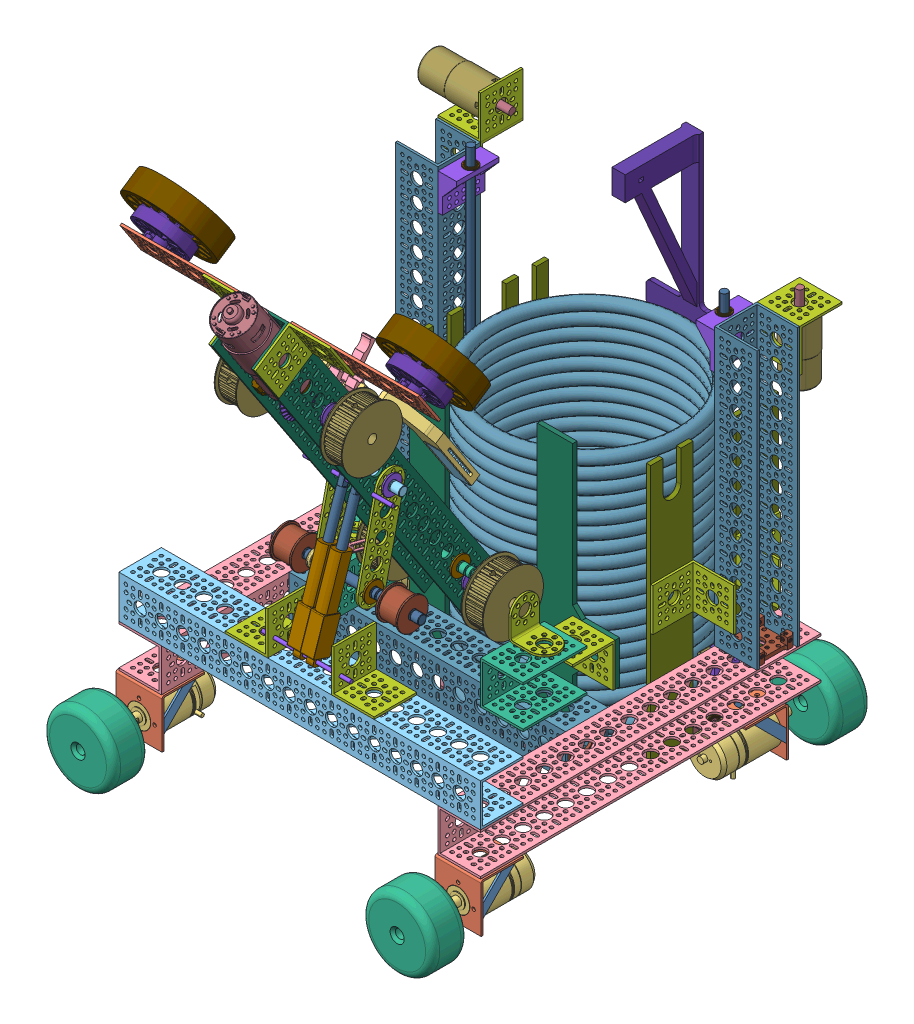
SolidWorks assembly 底座3.5, configuration 默认. Lengths in mm.
Overall size (466.71 646.3 560.79).
166 component instances, 54 part files, 189 mates.
Components (placement in the parent):
- 电机连接支架-5: 电机连接支架 [默认] at (-222.052 128.3372 691.3695) x (0 0 1) z (-1 0 0) size (48 54.5 52)
  - 小兔电机连接支架02-1: 小兔电机连接支架02 [默认] at (-18.8303 11.0829 24.6066) size (36.21 36.21 2)
  - 小兔电机连接支架02-2: 小兔电机连接支架02 [默认] at (-18.8303 11.0829 -25.3934) size (36.21 36.21 2)
  - 小兔电机连接支架-1: 小兔电机连接支架 [默认] at (17.3829 -18.9171 0.6066) size (48 54.5 52)
- 电机连接支架-6: 电机连接支架 [默认] at (137.948 128.3372 691.3695) x (0 0 1) z (-1 0 0) size (48 54.5 52)
  - 小兔电机连接支架02-1: 小兔电机连接支架02 [默认] at (-18.8303 11.0829 24.6066) size (36.21 36.21 2)
  - 小兔电机连接支架02-2: 小兔电机连接支架02 [默认] at (-18.8303 11.0829 -25.3934) size (36.21 36.21 2)
  - 小兔电机连接支架-1: 小兔电机连接支架 [默认] at (17.3829 -18.9171 0.6066) size (48 54.5 52)
- 3508无刷电机带减速箱（00）-5: 3508无刷电机带减速箱（00） [默认] at (137.3414 109.4201 681.1524) x (-1 0 0) z (0 -1 0) size (42 98.3 47)
- 3508无刷电机带减速箱（00）-7: 3508无刷电机带减速箱（00） [默认] at (-222.6586 109.4201 681.1524) x (0 -1 0) z (1 0 0) size (42 98.3 47)
- 384mm-U型梁-1: 384mm-U型梁 [默认] at (-201.1586 165.4201 709.5024) x (0 -1 0) z (1 0 0) size (48 384 48)
- 384mm-U型梁-2: 384mm-U型梁 [默认] at (115.8414 165.4201 709.5024) x (0 1 0) z (-1 0 0) size (48 384 48)
- 408mm-U型梁-10: 408mm-U型梁 [默认] at (161.3414 213.4201 707.0024) x (0 1 0) z (0 0 1) size (48 408 48)
- 电机连接支架-7: 电机连接支架 [默认] at (136.7348 128.3372 383.6353) x (0 0 -1) z (1 0 0) size (48 54.5 52)
  - 小兔电机连接支架02-1: 小兔电机连接支架02 [默认] at (-18.8303 11.0829 24.6066) size (36.21 36.21 2)
  - 小兔电机连接支架02-2: 小兔电机连接支架02 [默认] at (-18.8303 11.0829 -25.3934) size (36.21 36.21 2)
  - 小兔电机连接支架-1: 小兔电机连接支架 [默认] at (17.3829 -18.9171 0.6066) size (48 54.5 52)
- 3508无刷电机带减速箱（00）-8: 3508无刷电机带减速箱（00） [默认] at (137.3414 109.4201 393.8524) x (1 0 0) z (0 -1 0) size (42 98.3 47)
- 电机连接支架-8: 电机连接支架 [默认] at (-223.2652 128.3372 383.6353) x (0 0 -1) z (1 0 0) size (48 54.5 52)
  - 小兔电机连接支架02-1: 小兔电机连接支架02 [默认] at (-18.8303 11.0829 24.6066) size (36.21 36.21 2)
  - 小兔电机连接支架02-2: 小兔电机连接支架02 [默认] at (-18.8303 11.0829 -25.3934) size (36.21 36.21 2)
  - 小兔电机连接支架-1: 小兔电机连接支架 [默认] at (17.3829 -18.9171 0.6066) size (48 54.5 52)
- 3508无刷电机带减速箱（00）-9: 3508无刷电机带减速箱（00） [默认] at (-222.6586 109.4201 393.8524) x (1 0 0) z (0 -1 0) size (42 98.3 47)
- 麦轮（临时）-1: 麦轮（临时） [默认] at (-222.6586 109.4201 324.5024) x (0 0 -1) z (0.996866 -0.079106 0) size (40 80 80)
- 麦轮（临时）-2: 麦轮（临时） [默认] at (137.3414 109.4201 324.5024) x (0 0 -1) z (0.923265 -0.384164 0) size (40 80 80)
- 麦轮（临时）-3: 麦轮（临时） [默认] at (137.3414 109.4201 779.5024) x (0 0 -1) z (0.99707 -0.076496 0) size (40 80 80)
- 麦轮（临时）-4: 麦轮（临时） [默认] at (-222.6586 109.4201 779.5024) x (0 0 -1) z (0.996866 -0.079106 0) size (40 80 80)
- 48x48-L形支架-3: 48x48-L形支架 [默认] at (-81.1586 261.4201 709.5024) x (0 -1 0) z (1 0 0) size (48 48 48)
- 48x48-L形支架-4: 48x48-L形支架 [默认] at (-4.1586 261.4201 661.5024) x (0 -1 0) z (-1 0 0) size (48 48 48)
- 升降轴-1: 升降轴 [默认] at (-92.6586 252.9349 701.0171) x (1 0 0) z (0 0.719401 -0.694595) size (100 4 4)
- 电动推杆01-1: 电动推杆01 [默认] at (-54.1586 252.9349 701.0171) x (1 0 0) z (0 -0.94837 0.317167) size (15 20 103)
- 电动推杆01-2: 电动推杆01 [默认] at (-39.1586 252.9349 701.0171) x (1 0 0) z (0 -0.94837 0.317167) size (15 20 103)
- 电动推杆2-1: 电动推杆2 [默认] at (-35.1586 340.9577 671.5793) x (-1 0 0) z (0 -0.317167 -0.94837) size (9 66 9)
- 电动推杆2-2: 电动推杆2 [默认] at (-50.1586 340.9577 671.5793) x (-1 0 0) z (0 -0.317167 -0.94837) size (9 66 9)
- 升降轴-2: 升降轴 [默认] at (-94.6586 399.2825 652.0735) x (1 0 0) z (0 -0.677442 -0.735576) size (100 4 4)
- 电机转向座-9: 电机转向座 [默认] at (137.3414 189.4201 373.5024) x (0 0 -1) z (1 0 0) size (43.24 12.23 43.24)
- 电机转向座-12: 电机转向座 [默认] at (-222.6586 189.4201 373.5024) x (0 0 -1) z (1 0 0) size (43.24 12.23 43.24)
- 48x48-L形支架-17: 48x48-L形支架 [默认] at (161.3414 477.4201 347.0024) x (0 1 0) z (0 0 1) size (48 48 48)
- 48x48-L形支架-18: 48x48-L形支架 [默认] at (-198.6586 477.4201 347.0024) x (0 1 0) z (0 0 1) size (48 48 48)
- 一级摩擦轮电机01-2: 一级摩擦轮电机01 [默认] at (137.3414 425.6201 325.5024) x (0.035714 0 0.999362) z (-0.999362 0 0.035714) size (36 73.3 36)
- 一级摩擦轮电机02-2: 一级摩擦轮电机02 [默认] at (137.3414 495.9201 325.5024) x (-0.966562 0 0.256432) z (-0.256432 0 -0.966562) size (8 20 8)
- 312mm-U型梁-7: 312mm-U型梁 [默认] at (-198.6586 186.9201 541.5024) x (0 0 1) z (0 1 0) size (48 312 48)
- 电机转向座-13: 电机转向座 [默认] at (113.3414 165.4201 541.5024) x (0 0 -1) z (0 1 0) size (43.24 12.23 43.24)
- 总装-2: 总装 [默认] at (-93.0333 217.2746 993.3883) x (-0.999953 0.009266 0.002717) z (0 0.281421 -0.959585) size (409.26 486.07 201.86)
  - 432mm-U型梁-1: 432mm-U型梁 [默认] at (-52.5612 -100.8788 473.6792) x (0.999953 -0.009656 0) z (0.002854 0.295554 0.955322) size (48 432 48)
  - 发射法兰1-2: 发射法兰1 [默认] at (95.3037 298.6557 389.1988) x (0.597612 -0.766469 0.235342) z (0.801781 0.57024 -0.178814) size (30 11 30)
  - 发射无刷电机-2: 发射无刷电机 [默认] at (95.2101 288.9616 357.8642) x (-0.009225 -0.955277 0.295568) z (-0.999953 0.009656 0) size (58.5 35.4 58.5)
  - 摩擦轮-2: 摩擦轮 [默认] at (94.6021 282.6082 387.0905) x (-0.954993 -0.28256 0.09027) z (-0.002854 -0.295554 -0.955322) size (96 96 24)
    - 摩擦轮.STEP-1: 摩擦轮.STEP [默认] at origin size (96 96 24)
      - 3613-0014-0096 Rubber.STEP-1: 3613-0014-0096 Rubber.STEP [默认] at (-5.0141 13.8433 -6.759) size (96 96 24)
      - 3613-0014-0096 Core.STEP-1: 3613-0014-0096 Core.STEP [默认] at (-5.0141 13.8433 -6.759) x (1 0 0) z (0 -1 0) size (35.2 24 35.2)
  - 5孔平板-2: 5孔平板 [默认] at (119.072 274.5458 384.7583) x (0.002854 0.295554 0.955322) z (-0.009225 -0.955277 0.295568) size (2.5 144 43)
  - 48x48-L形支架-2: 48x48-L形支架 [默认] at (-22.5815 259.3374 339.6418) x (0.002854 0.295554 0.955322) z (-0.999953 0.009656 0) size (48 48 48)
  - 装配体3-2: 装配体3 [默认] at (-128.0634 200.7559 231.0431) x (0.002854 0.295554 0.955322) z (0.999953 -0.009656 0) size (95.3 120.73 180.37)
    - 发射法兰1-1: 发射法兰1 [默认] at (180.6617 -48.8364 -65.5887) x (0 1 0) z (0 0 1) size (30 11 30)
    - 发射无刷电机-1: 发射无刷电机 [默认] at (147.8617 -48.8364 -65.5887) x (0 -1 0) z (0 0 1) size (58.5 35.4 58.5)
    - 摩擦轮-1: 摩擦轮 [默认] at (173.9027 -63.5495 -65.0421) x (0 -0.305413 0.95222) z (-1 0 0) size (96 96 24)
      - 摩擦轮.STEP-1: 摩擦轮.STEP [默认] at origin size (96 96 24)
        - 3613-0014-0096 Rubber.STEP-1: 3613-0014-0096 Rubber.STEP [默认] at (-5.0141 13.8433 -6.759) size (96 96 24)
        - 3613-0014-0096 Core.STEP-1: 3613-0014-0096 Core.STEP [默认] at (-5.0141 13.8433 -6.759) x (1 0 0) z (0 -1 0) size (35.2 24 35.2)
    - 5孔平板-1: 5孔平板 [默认] at (169.3617 -70.3364 -89.5887) x (1 0 0) z (0 -1 0) size (2.5 144 43)
    - 48x48-L形支架-1: 48x48-L形支架 [默认] at (121.3617 -72.8364 51.9113) size (48 48 48)
  - 2306-4008-0014 assembly-1: 2306-4008-0014 assembly [默认] at (-186.8079 96.5973 629.512) x (0 0.597801 0.801645) z (-0.223733 -0.781323 0.582647)
  - 不锈钢花篮螺丝-02-1: 不锈钢花篮螺丝-02 [默认] at (-13.6983 -11.7016 355.7521) x (-0.999953 0.009656 0) z (0.008275 0.856874 0.51546) size (4.31 46.15 18.3)
  - 花篮螺丝-1: 花篮螺丝 [默认] at (-71.9313 -35.5534 412.0649) x (0.008275 0.856874 0.51546) z (0.999953 -0.009656 0) size (18.3 77.15 7)
    - 不锈钢花篮螺丝-01-1: 不锈钢花篮螺丝-01 [默认] at (-8.1072 20.254 58) size (9 58 7)
    - 不锈钢花篮螺丝-02-1: 不锈钢花篮螺丝-02 [默认] at (-8.1072 29.254 58) x (0 0 1) z (1 0 0) size (4.31 46.15 18.3)
  - 张紧固定轴2-1: 张紧固定轴2 [默认] at (-22.3528 75.9048 396.3908) x (-0.999953 0.009656 0) z (0.003811 0.394647 0.918825) size (81 10 10)
  - 张紧固定轴3-1: 张紧固定轴3 [默认] at (-78.1786 -61.1289 438.9525) x (0.999953 -0.009656 0) z (-0.003263 -0.337938 -0.941163) size (90 10 10)
  - 圆角孔板5孔(1)-1: 圆角孔板5孔(1) [默认] at (-25.1629 -7.9825 349.7537) x (0.00844 0.874027 0.485803) z (-0.004691 -0.485781 0.874068) size (128 2.5 32)
  - 铜套-1: 铜套 [默认] at (-22.3528 75.9048 396.3908) x (-0.999953 0.009656 0) z (0.009537 0.98756 -0.156954) size (10 22 22)
  - 铜套1-5: 铜套1 [默认] at (-78.1786 -61.1289 438.9525) x (0.999953 -0.009656 0) z (0 0 1) size (10 22 22)
  - 铜套1-6: 铜套1 [默认] at (-26.181 -61.631 438.9525) x (-0.999953 0.009656 0) z (0 0 1) size (10 22 22)
  - 张紧固定轴(中)-1: 张紧固定轴(中) [默认] at (-77.6605 -7.4756 349.7537) x (0.999953 -0.009656 0) z (0.007656 0.792843 0.609378) size (166 10 10)
  - 张紧轮1-3: 张紧轮1 [默认] at (-4.1639 -8.1853 349.7537) x (0.999953 -0.009656 0) z (-0.000665 -0.068842 0.997627) size (25 35 35)
  - 铜套1-8: 铜套1 [默认] at (-23.163 -8.0018 349.7537) x (-0.999953 0.009656 0) z (-0.007437 -0.770127 -0.637848) size (10 22 22)
  - 同步轮四十齿(1)-1: 同步轮四十齿(1) [默认] at (20.0954 -85.0067 446.0461) x (0.009586 0.99273 -0.119983) z (0.001159 0.119977 0.992776) size (68 25 68)
  - 同步轮四十齿(1)-2: 同步轮四十齿(1) [默认] at (22.7522 190.1132 360.9227) x (0.004551 0.471293 -0.881965) z (0.008516 0.881924 0.471315) size (68 25 68)
  - 同步轮四十齿(1)-3: 同步轮四十齿(1) [默认] at (-99.1635 -83.855 446.0461) x (0.009623 0.996484 -0.083229) z (0.000804 0.083225 0.99653) size (68 25 68)
  - 同步轮四十齿(1)-4: 同步轮四十齿(1) [默认] at (-96.5067 191.2649 360.9227) x (0.00965 0.999279 0.036717) z (-0.000355 -0.036715 0.999326) size (68 25 68)
  - 皮带电机装配体-3: 皮带电机装配体 [默认] at (17.3534 305.199 468.5412) x (0.009225 0.955277 -0.295568) z (0.002854 0.295554 0.955322) size (182.3 67.11 64.42)
    - 发射轮电机1-1: 发射轮电机1 [默认] at (-31.948 68.6302 -206.7966) size (148.5 67.11 64.42)
    - 3204-0002-0002 assembly-1: 3204-0002-0002 assembly [默认] at (-82.9257 129.4143 -179.1986) x (0 1 0) z (0 0 1) size (28.67 52.38 42.6)
      - 2306-4008-0014 assembly(2)-1: 2306-4008-0014 assembly(2) [默认] at (-86.5036 -22.1715 14.0673) x (0 1 0) z (-0.223733 0 0.97465) size (15.4 23.81 24.42)
        - 2306-4008-0014-1: 2306-4008-0014 [默认] at (-4.2928 -28.4802 22.5212) size (15.32 23.81 24.42)
        - 2306-4008-0014 clamp-1: 2306-4008-0014 clamp [默认] at (-4.2932 -28.4802 22.5212) size (9.55 8.86 18.72)
        - 2800-0004-0012_90128A207-1: 2800-0004-0012_90128A207 [默认] at (-8.9015 -37.2302 16.6212) x (0.549526 0 0.835476) z (0 -1 0) size (7 7 16.17)
        - 2800-0004-0012_90128A207-2: 2800-0004-0012_90128A207 [默认] at (-8.9015 -37.2302 28.4212) x (0.549526 0 -0.835476) z (0 -1 0) size (7 7 16.17)
      - 2307-0014-0028-1: 2307-0014-0028 [默认] at (-76.6728 -4.8452 42.3896) size (6.41 42.6 42.6)
    - 齿轮组法兰-1: 齿轮组法兰 [默认] at (-78.0805 56.1302 -136.809) x (0 1 0) z (0 0 1) size (12 30 30) (hidden)
    - 电机转向座1-1: 电机转向座1 [默认] at (-41.0801 65.9902 -136.809) x (0 0 -1) z (0 -1 0) size (43.24 12.23 43.24)
  - 张紧轮1-4: 张紧轮1 [默认] at (-124.1583 -7.0266 349.7537) x (0.999953 -0.009656 0) z (-0.001384 -0.14335 0.989671) size (25 35 35)
  - 滑轨9-1: 滑轨9 [默认] at (-54.9831 -92.7733 473.7957) x (0.999953 -0.009656 0) z (-0.009225 -0.955277 0.295568) size (5 3.7 400)
  - 钩子总装修改-1: 钩子总装修改 [默认] at (-51.1458 183.362 391.6503) x (0.999953 -0.009656 0) z (-0.009225 -0.955277 0.295568) size (146 51.58 153.26)
    - 滑块1-1: 滑块1 [默认] at (1.3294 2.8515 16) size (12 5 16)
    - 滑块座1-1: 滑块座1 [默认] at (-33.6706 2.8515 4) size (146 18 125)
    - 抓钩1-1: 抓钩1 [默认] at (6.3294 45.8627 -7.2454) x (0 -0.424487 0.905434) z (0 -0.905434 -0.424487) size (35.49 30 38.32)
    - 移动块-1: 移动块 [默认] at (62.3294 9.8515 101.6458) x (0 0 1) z (-1 0 0) size (60 11 18)
    - 移动块-2: 移动块 [默认] at (-59.6706 9.8515 101.6458) x (0 0 1) z (-1 0 0) size (60 11 18)
  - 铜套-2: 铜套 [默认] at (-75.7432 191.0643 360.9227) x (0.999953 -0.009656 0) z (0 0 1) size (10 22 22)
  - 铜套-3: 铜套 [默认] at (-23.7457 190.5622 360.9227) x (-0.999953 0.009656 0) z (-0.009078 -0.94012 -0.340724) size (10 22 22)
  - 铜套-4: 铜套 [默认] at (-78.4 -84.0555 446.0461) x (0.999953 -0.009656 0) z (0.000026 0.002689 0.999996) size (10 22 22)
  - 铜套-5: 铜套 [默认] at (-26.4024 -84.5576 446.0461) x (-0.999953 0.009656 0) z (-0.009078 -0.94012 -0.340724) size (10 22 22)
  - 铜套-6: 铜套 [默认] at (-79.3501 76.4552 396.3908) x (0.999953 -0.009656 0) z (0 0 1) size (10 22 22)
  - 圆角孔板5孔(1)-2: 圆角孔板5孔(1) [默认] at (-75.6606 -7.4949 349.7537) x (0.00844 0.874027 0.485803) z (-0.004691 -0.485781 0.874068) size (128 2.5 32)
  - 铜套1-9: 铜套1 [默认] at (-80.1604 -7.4514 349.7537) x (0.999953 -0.009656 0) z (0.003758 0.38916 -0.921163) size (10 22 22)
- 72mm-U型梁-5: 72mm-U型梁 [默认] at (43.8414 213.4201 517.5024) x (0 -1 0) z (-1 0 0) size (48 72 48)
- 72mm-U型梁-6: 72mm-U型梁 [默认] at (-129.1586 213.4201 517.5024) x (0 1 0) z (1 0 0) size (48 72 48)
- 圆角90°法兰-7: 圆角90°法兰 [默认] at (41.3414 237.4201 541.5024) x (1 0 0) z (0 -1 0) size (40 32 40)
- 圆角90°法兰-8: 圆角90°法兰 [默认] at (-126.6586 237.4201 541.5024) x (-1 0 0) z (0 -1 0) size (40 32 40)
- 轴承座-1: 轴承座 [Default] at (113.3414 492.4201 397.5024) x (-1 0 0) z (0 0 -1) size (21 41 48)
- 8-14轴承-7: 8-14轴承 [默认] at (100.3414 493.4201 373.5024) x (0.974446 0 0.224624) z (-0.224624 0 0.974446) size (15 5 15)
- 轴承座-2: 轴承座 [Default] at (113.3414 150.4201 349.5024) x (-1 0 0) z (0 0 1) size (21 41 48)
- 8-14轴承-8: 8-14轴承 [默认] at (100.3414 146.4201 373.5024) x (0.983901 0 0.178713) z (-0.178713 0 0.983901) size (15 5 15)
- 螺纹杆-3: 螺纹杆 [默认] at (100.3414 117.4201 373.5024) x (0.005803 0 0.999983) z (-0.999983 0 0.005803) size (8 400 8)
- 切边螺纹滑块-1: 切边螺纹滑块 [Default] at (100.3414 168.0411 373.5024) x (-1 0 0) z (0 0 1) size (10.2 15 22)
- 轴承座-3: 轴承座 [Default] at (-198.6586 492.4201 349.5024) size (21 41 48)
- 轴承座-4: 轴承座 [Default] at (-198.6586 150.4201 397.5024) x (1 0 0) z (0 0 -1) size (21 41 48)
- 8-14轴承-9: 8-14轴承 [默认] at (-185.6586 493.4201 373.5024) size (15 5 15)
- 8-14轴承-10: 8-14轴承 [默认] at (-185.6586 146.4201 373.5024) size (15 5 15)
- 螺纹杆-4: 螺纹杆 [默认] at (-185.6586 117.4201 373.5024) x (0.186577 0 0.98244) z (-0.98244 0 0.186577) size (8 400 8)
- 切边螺纹滑块-2: 切边螺纹滑块 [Default] at (-185.6586 168.0411 373.5024) x (-1 0 0) z (0 0 1) size (10.2 15 22)
- 转换块-1: 转换块 [Default] at (100.3414 158.0411 373.5024) x (0 0 1) z (-1 0 0) size (24 85 26)
- 转换块-2: 转换块 [Default] at (-185.6586 158.0411 373.5024) x (0 0 -1) z (1 0 0) size (24 85 26)
- 312mm-U型梁-8: 312mm-U型梁 [默认] at (115.8414 501.4201 373.5024) x (0 0 -1) z (-1 0 0) size (48 312 48)
- 312mm-U型梁-9: 312mm-U型梁 [默认] at (-201.1586 501.4201 373.5024) x (0 0 1) z (1 0 0) size (48 312 48)
- 8-14轴承-11: 8-14轴承 [默认] at (83.3414 90.0411 373.5024) x (0 0.99609 -0.088349) z (0 -0.088349 -0.99609) size (15 5 15)
- 8-14轴承-12: 8-14轴承 [默认] at (-168.6586 90.0411 373.5024) x (0 -0.55352 0.832836) z (0 -0.832836 -0.55352) size (15 5 15)
- 铲板-1: 铲板 [Default] at (-42.6586 74.7848 398.3468) x (-1 0 0) z (0 0.010285 -0.999947) size (262 29 178.51)
- 20个环-3: 20个环 [Default] at (-127.5441 -59.6219 226.4779) size (229.8 290.93 229.39)
  - 圆环-1: 圆环 [默认] at (-22.7884 145.7519 157.2951) size (228 14 228)
  - 圆环-2: 圆环 [默认] at (-23.1175 159.9955 157.1344) size (228 14 228)
  - 圆环-3: 圆环 [默认] at (-23.0314 188.5505 156.9811) size (228 14 228)
  - 圆环-4: 圆环 [默认] at (-22.9968 174.3685 156.6405) size (228 14 228)
  - 圆环-5: 圆环 [默认] at (-23.8175 218.055 156.8293) size (228 14 228)
  - 圆环-6: 圆环 [默认] at (-23.491 232.7117 157.4697) size (228 14 228)
  - 圆环-7: 圆环 [默认] at (-24.5846 203.4176 157.6394) size (228 14 228)
  - 圆环-8: 圆环 [默认] at (-22.9081 247.4608 157.3208) size (228 14 228)
  - 圆环-9: 圆环 [默认] at (-23.5661 364.5462 157.293) size (228 14 228)
  - 圆环-10: 圆环 [默认] at (-23.6099 320.9711 157.4866) size (228 14 228)
  - 圆环-11: 圆环 [默认] at (-23.6825 350.1705 157.5218) size (228 14 228)
  - 圆环-12: 圆环 [默认] at (-24.0088 276.7124 157.1259) size (228 14 228)
  - 圆环-13: 圆环 [默认] at (-23.8881 291.321 157.9228) size (228 14 228)
  - 圆环-14: 圆环 [默认] at (-23.6797 261.8797 158.031) size (228 14 228)
  - 圆环-15: 圆环 [默认] at (-24.0091 335.4434 157.9465) size (228 14 228)
  - 圆环-16: 圆环 [默认] at (-23.4562 306.0805 156.7976) size (228 14 228)
  - 圆环-17: 圆环 [默认] at (-24.0369 393.8042 157.2623) size (228 14 228)
  - 圆环-18: 圆环 [默认] at (-23.9162 408.195 157.1866) size (228 14 228)
  - 圆环-19: 圆环 [默认] at (-23.9606 379.2206 157.4915) size (228 14 228)
  - 圆环-20: 圆环 [默认] at (-23.698 422.6814 157.0029) size (228 14 228)
- 48x48-L形支架-20: 48x48-L形支架 [默认] at (-134.6586 232.4201 517.5024) x (0 0 -1) z (0 1 0) size (48 48 48)
- 前挡板-1: 前挡板 [Default] at (-94.6586 402.9201 493.5024) x (-1 0 0) z (0 0 -1) size (88 278 5)
- 48x48-L形支架-22: 48x48-L形支架 [默认] at (-198.6586 261.4201 400.0024) x (1 0 0) z (0 0 -1) size (48 48 48)
- 48x48-L形支架-23: 48x48-L形支架 [默认] at (-198.6586 213.4201 347.0024) size (48 48 48)
- 侧挡板-1: 侧挡板 [Default] at (-174.6586 77.4201 301.5024) x (0 0 1) z (1 0 0) size (48 300 5)
- 侧挡板-2: 侧挡板 [Default] at (-174.6586 77.4201 397.5024) x (0 0 1) z (1 0 0) size (48 300 5)
- 侧挡板-3: 侧挡板 [Default] at (84.3414 77.4201 301.5024) x (0 0 1) z (1 0 0) size (48 300 5)
- 侧挡板-4: 侧挡板 [Default] at (84.3414 77.4201 397.5024) x (0 0 1) z (1 0 0) size (48 300 5)
- 48x48-L形支架-24: 48x48-L形支架 [默认] at (91.8414 213.4201 325.5024) x (0 0 1) z (-1 0 0) size (48 48 48)
- 48x48-L形支架-25: 48x48-L形支架 [默认] at (113.3414 213.4201 400.0024) x (-1 0 0) z (0 0 -1) size (48 48 48)
- 48x48-L形支架-26: 48x48-L形支架 [默认] at (97.3414 232.4201 517.5024) x (0 0 -1) z (0 1 0) size (48 48 48)
- 前挡板-2: 前挡板 [Default] at (9.3414 402.9201 488.5024) size (88 278 5)
- 推板-1: 推板 [默认] at (-41.8089 369.725 264.6148) size (100 195 86)
- 一级摩擦轮电机02-3: 一级摩擦轮电机02 [默认] at (-206.7756 525.4201 325.5024) x (0 -0.907269 -0.420551) z (0 -0.420551 0.907269) size (8 20 8)
- 一级摩擦轮电机01-4: 一级摩擦轮电机01 [默认] at (-277.0756 525.4201 325.5024) x (0 -0.562838 0.826567) z (0 0.826567 0.562838) size (36 73.3 36)
- 48x48-L形支架-27: 48x48-L形支架 [默认] at (-201.1586 525.4201 349.5024) x (0 -1 0) z (1 0 0) size (48 48 48)
Mates (geometry in assembly coordinates):
- Coincident37: coincident anti-aligned: plane of 电机连接支架-5/小兔电机连接支架-1 through (-222.6586 109.4201 708.7524) normal (0 0 -1); plane of 3508无刷电机带减速箱（00）-7 through (-222.6586 96.4201 708.7524) normal (0 0 1)
- Concentric38: concentric aligned: cylinder of 电机连接支架-5/小兔电机连接支架-1 through (-222.6586 109.4201 710.7524) axis (0 0 -1) radius 13.25; cylinder of 3508无刷电机带减速箱（00）-7 through (-222.6586 109.4201 672.4524) axis (0 0 -1) radius 13
- Concentric39: concentric anti-aligned: cylinder of 电机连接支架-5/小兔电机连接支架-1 through (-222.6586 126.9201 710.7524) axis (0 0 -1) radius 2; cylinder of 3508无刷电机带减速箱（00）-7 through (-222.6586 126.9201 708.7524) axis (0 0 1) radius 1.65
- Coincident38: coincident anti-aligned: plane of 电机连接支架-6/小兔电机连接支架-1 through (137.3414 109.4201 708.7524) normal (0 0 -1); plane of 3508无刷电机带减速箱（00）-5 through (124.3414 109.4201 708.7524) normal (0 0 1)
- Concentric40: concentric aligned: cylinder of 电机连接支架-6/小兔电机连接支架-1 through (137.3414 109.4201 710.7524) axis (0 0 -1) radius 13.25; cylinder of 3508无刷电机带减速箱（00）-5 through (137.3414 109.4201 672.4524) axis (0 0 -1) radius 13
- Concentric41: concentric anti-aligned: cylinder of 电机连接支架-6/小兔电机连接支架-1 through (137.3414 126.9201 710.7524) axis (0 0 -1) radius 2; cylinder of 3508无刷电机带减速箱（00）-5 through (137.3414 126.9201 708.7524) axis (0 0 1) radius 1.65
- Concentric261: concentric anti-aligned: cylinder of 384mm-U型梁-2 through (137.3414 179.4201 685.5024) axis (0 1 0) radius 7; cylinder of 408mm-U型梁-10 through (137.3414 199.4201 685.5024) axis (0 -1 0) radius 7
- Concentric262: concentric anti-aligned: cylinder of 384mm-U型梁-1 through (-222.6586 179.4201 685.5024) axis (0 1 0) radius 7; cylinder of 408mm-U型梁-10 through (-222.6586 199.4201 685.5024) axis (0 -1 0) radius 7
- Coincident94: coincident aligned: plane of 384mm-U型梁-2 through (161.3414 186.9201 325.5024) normal (1 0 0); plane of 408mm-U型梁-10 through (161.3414 213.4201 707.0024) normal (1 0 0)
- Coincident95: coincident aligned: plane of 384mm-U型梁-1 through (-246.6586 186.9201 325.5024) normal (-1 0 0); plane of 408mm-U型梁-10 through (-246.6586 213.4201 707.0024) normal (-1 0 0)
- Coincident96: coincident anti-aligned: plane of 384mm-U型梁-1 through (-246.6586 189.4201 325.5024) normal (0 1 0); plane of 408mm-U型梁-10 through (-246.6586 189.4201 661.5024) normal (0 -1 0)
- Coincident97: coincident anti-aligned: plane of 384mm-U型梁-2 through (161.3414 189.4201 325.5024) normal (0 1 0); plane of 408mm-U型梁-10 through (-246.6586 189.4201 661.5024) normal (0 -1 0)
- Concentric267: concentric aligned: cylinder of 电机连接支架-7/小兔电机连接支架-1 through (137.3414 109.4201 364.2524) axis (0 0 1) radius 13.25; cylinder of 3508无刷电机带减速箱（00）-8 through (137.3414 109.4201 402.5524) axis (0 0 1) radius 13
- Coincident104: coincident anti-aligned: plane of 电机连接支架-7/小兔电机连接支架-1 through (137.3414 109.4201 366.2524) normal (0 0 1); plane of 3508无刷电机带减速箱（00）-8 through (150.3414 109.4201 366.2524) normal (0 0 -1)
- Concentric268: concentric anti-aligned: cylinder of 电机连接支架-7/小兔电机连接支架-1 through (137.3414 126.9201 364.2524) axis (0 0 1) radius 2; cylinder of 3508无刷电机带减速箱（00）-8 through (137.3414 126.9201 366.2524) axis (0 0 -1) radius 1.65
- Concentric269: concentric aligned: cylinder of 电机连接支架-8/小兔电机连接支架-1 through (-222.6586 109.4201 364.2524) axis (0 0 1) radius 13.25; cylinder of 3508无刷电机带减速箱（00）-9 through (-222.6586 109.4201 402.5524) axis (0 0 1) radius 13
- Coincident105: coincident anti-aligned: plane of 电机连接支架-8/小兔电机连接支架-1 through (-222.6586 109.4201 366.2524) normal (0 0 1); plane of 3508无刷电机带减速箱（00）-9 through (-209.6586 109.4201 366.2524) normal (0 0 -1)
- Concentric270: concentric anti-aligned: cylinder of 电机连接支架-8/小兔电机连接支架-1 through (-222.6586 126.9201 364.2524) axis (0 0 1) radius 2; cylinder of 3508无刷电机带减速箱（00）-9 through (-222.6586 126.9201 366.2524) axis (0 0 -1) radius 1.65
- Concentric271: concentric anti-aligned: cylinder of 电机连接支架-6/小兔电机连接支架-1 through (137.3414 86.9201 685.5024) axis (0 1 0) radius 7; cylinder of 384mm-U型梁-2 through (137.3414 151.4201 685.5024) axis (0 -1 0) radius 7
- Coincident106: coincident anti-aligned: plane of 电机连接支架-6/小兔电机连接支架-1 through (163.3414 141.4201 662.7524) normal (0 1 0); plane of 384mm-U型梁-2 through (161.3414 141.4201 325.5024) normal (0 -1 0)
- Concentric272: concentric anti-aligned: cylinder of 电机连接支架-6/小兔电机连接支架-1 through (153.3414 86.9201 701.5024) axis (0 1 0) radius 2; cylinder of 384mm-U型梁-2 through (153.3414 151.4201 701.5024) axis (0 -1 0) radius 2
- Concentric273: concentric anti-aligned: cylinder of 电机连接支架-5/小兔电机连接支架-1 through (-222.6586 86.9201 685.5024) axis (0 1 0) radius 7; cylinder of 384mm-U型梁-1 through (-222.6586 151.4201 685.5024) axis (0 -1 0) radius 7
- Coincident107: coincident anti-aligned: plane of 电机连接支架-5/小兔电机连接支架-1 through (-196.6586 141.4201 662.7524) normal (0 1 0); plane of 384mm-U型梁-1 through (-246.6586 141.4201 325.5024) normal (0 -1 0)
- Concentric274: concentric anti-aligned: cylinder of 电机连接支架-5/小兔电机连接支架-1 through (-206.6586 86.9201 701.5024) axis (0 1 0) radius 2; cylinder of 384mm-U型梁-1 through (-206.6586 151.4201 701.5024) axis (0 -1 0) radius 2
- Coincident108: coincident anti-aligned: plane of 384mm-U型梁-2 through (161.3414 141.4201 325.5024) normal (0 -1 0); plane of 电机连接支架-7/小兔电机连接支架-1 through (111.3414 141.4201 412.2524) normal (0 1 0)
- Concentric276: concentric anti-aligned: cylinder of 384mm-U型梁-2 through (153.3414 151.4201 373.5024) axis (0 -1 0) radius 2; cylinder of 电机连接支架-7/小兔电机连接支架-1 through (153.3414 86.9201 373.5024) axis (0 1 0) radius 2
- Concentric277: concentric anti-aligned: cylinder of 384mm-U型梁-2 through (121.3414 151.4201 373.5024) axis (0 -1 0) radius 2; cylinder of 电机连接支架-7/小兔电机连接支架-1 through (121.3414 86.9201 373.5024) axis (0 1 0) radius 2
- Coincident109: coincident anti-aligned: plane of 384mm-U型梁-1 through (-246.6586 141.4201 325.5024) normal (0 -1 0); plane of 电机连接支架-8/小兔电机连接支架-1 through (-248.6586 141.4201 412.2524) normal (0 1 0)
- Concentric278: concentric anti-aligned: cylinder of 384mm-U型梁-1 through (-238.6586 151.4201 373.5024) axis (0 -1 0) radius 2; cylinder of 电机连接支架-8/小兔电机连接支架-1 through (-238.6586 86.9201 373.5024) axis (0 1 0) radius 2
- Concentric279: concentric anti-aligned: cylinder of 384mm-U型梁-1 through (-206.6586 151.4201 373.5024) axis (0 -1 0) radius 2; cylinder of 电机连接支架-8/小兔电机连接支架-1 through (-206.6586 86.9201 373.5024) axis (0 1 0) radius 2
- Concentric280: concentric anti-aligned: cylinder of 3508无刷电机带减速箱（00）-9 through (-222.6586 109.4201 402.5524) axis (0 0 1) radius 5; cylinder of 麦轮（临时）-1 through (-222.6586 109.4201 324.5024) axis (0 0 -1) radius 5
- Distance1: distance = 1 mm anti-aligned: plane of 麦轮（临时）-1 through (-222.6586 109.4201 324.5024) normal (0 0 1); plane of 384mm-U型梁-1 through (-201.1586 165.4201 325.5024) normal (0 0 -1)
- Concentric281: concentric anti-aligned: cylinder of 3508无刷电机带减速箱（00）-8 through (137.3414 109.4201 402.5524) axis (0 0 1) radius 5; cylinder of 麦轮（临时）-2 through (137.3414 109.4201 324.5024) axis (0 0 -1) radius 5
- Distance2: distance = 1 mm anti-aligned: plane of 384mm-U型梁-2 through (115.8414 165.4201 325.5024) normal (0 0 -1); plane of 麦轮（临时）-2 through (137.3414 109.4201 324.5024) normal (0 0 1)
- Concentric282: concentric aligned: cylinder of 3508无刷电机带减速箱（00）-5 through (137.3414 109.4201 672.4524) axis (0 0 -1) radius 5; cylinder of 麦轮（临时）-3 through (137.3414 109.4201 779.5024) axis (0 0 -1) radius 5
- Distance3: distance = 495 mm anti-aligned: plane of 麦轮（临时）-3 through (137.3414 109.4201 779.5024) normal (0 0 1); plane of 麦轮（临时）-2 through (137.3414 109.4201 284.5024) normal (0 0 -1)
- Concentric283: concentric aligned: cylinder of 3508无刷电机带减速箱（00）-7 through (-222.6586 109.4201 672.4524) axis (0 0 -1) radius 5; cylinder of 麦轮（临时）-4 through (-222.6586 109.4201 779.5024) axis (0 0 -1) radius 5
- Distance4: distance = 495 mm anti-aligned: plane of 麦轮（临时）-4 through (-222.6586 109.4201 779.5024) normal (0 0 1); plane of 麦轮（临时）-1 through (-222.6586 109.4201 284.5024) normal (0 0 -1)
- Coincident120: coincident anti-aligned: plane of 408mm-U型梁-10 through (-246.6586 237.4201 661.5024) normal (0 1 0); plane of 48x48-L形支架-3 through (-126.6586 237.4201 661.5024) normal (0 -1 0)
- Concentric309: concentric anti-aligned: cylinder of 408mm-U型梁-10 through (-102.6586 227.4201 685.5024) axis (0 1 0) radius 7; cylinder of 48x48-L形支架-3 through (-102.6586 247.4201 685.5024) axis (0 -1 0) radius 7
- Concentric310: concentric anti-aligned: cylinder of 408mm-U型梁-10 through (-118.6586 227.4201 669.5024) axis (0 1 0) radius 2; cylinder of 48x48-L形支架-3 through (-118.6586 247.4201 669.5024) axis (0 -1 0) radius 2
- Concentric311: concentric anti-aligned: cylinder of 408mm-U型梁-10 through (17.3414 227.4201 685.5024) axis (0 1 0) radius 7; cylinder of 48x48-L形支架-4 through (17.3414 247.4201 685.5024) axis (0 -1 0) radius 7
- Coincident121: coincident anti-aligned: plane of 408mm-U型梁-10 through (-246.6586 237.4201 661.5024) normal (0 1 0); plane of 48x48-L形支架-4 through (41.3414 237.4201 709.5024) normal (0 -1 0)
- Concentric312: concentric anti-aligned: cylinder of 408mm-U型梁-10 through (1.3414 227.4201 701.5024) axis (0 1 0) radius 2; cylinder of 48x48-L形支架-4 through (1.3414 247.4201 701.5024) axis (0 -1 0) radius 2
- Concentric313: concentric anti-aligned: cylinder of 48x48-L形支架-3 through (-88.6586 252.9349 701.0171) axis (1 0 0) radius 2; cylinder of 升降轴-1 through (7.3414 252.9349 701.0171) axis (-1 0 0) radius 2
- Distance6: distance = 11.5 mm aligned: plane of 升降轴-1 through (-92.6586 252.9349 701.0171) normal (-1 0 0); plane of 48x48-L形支架-3 through (-81.1586 282.9201 661.5024) normal (-1 0 0)
